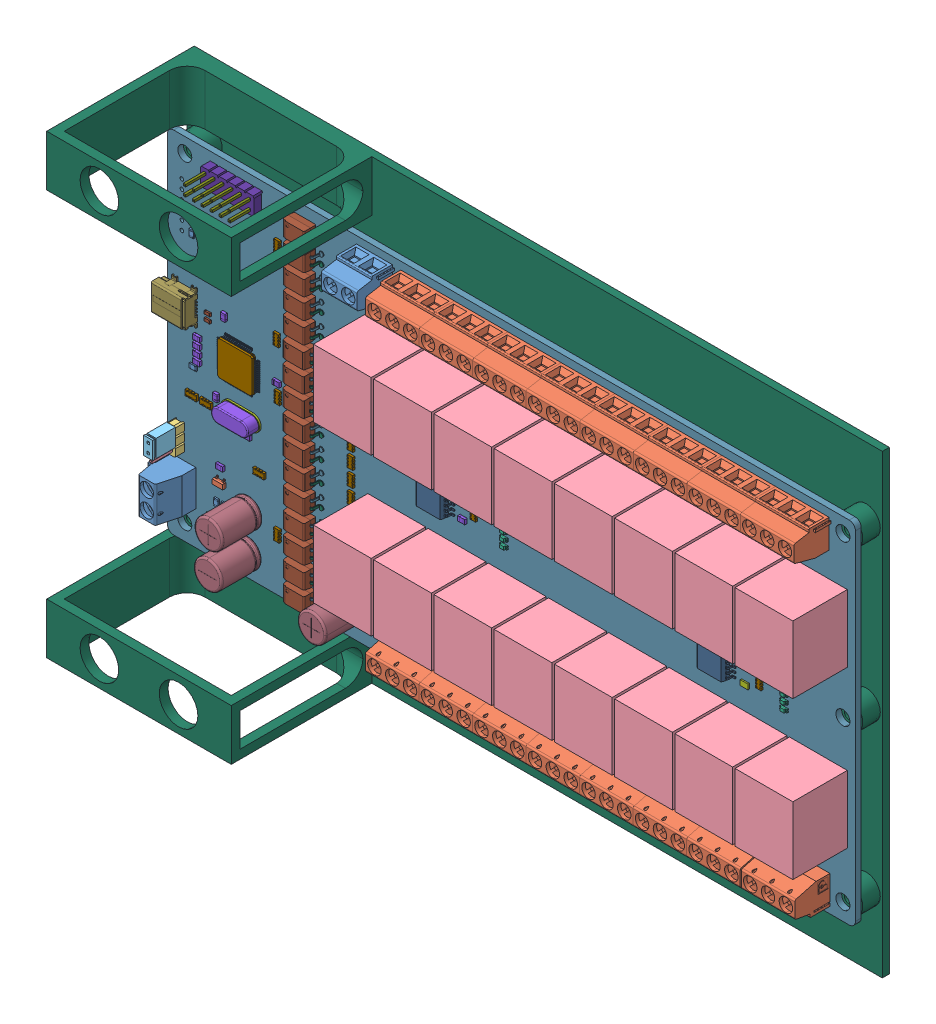
SolidWorks assembly Assem2, configuration Default. Lengths in mm.
Overall size (201.04 129.82 42).
600 component instances, 33 part files, 0 mates.
Components (placement in the parent):
- 16_Channel_USB_Relay.step-1: 16_Channel_USB_Relay.step [Default] at (-11.9082 58.988 141.1455) size (200.04 103.47 20)
  - X277.step-1: X277.step [Default] at origin size (10.73 8.1 13.5)
    - 1729128_07.step-1: 1729128_07.step [Default] at (64.7474 97.3538 0) x (0 1 0) z (1 0 0) size (8.1 13.5 10.73)
      - mkdsn_1.5-2-5.08.step-1: mkdsn_1.5-2-5.08.step [Default] at (-39.331 -15.5089 -8.19) x (-1 0 0) z (0 0 -1) size (8.1 13.5 10.73)
  - X276.step-1: X276.step [Default] at origin size (15.81 8.1 13.5)
    - 1729131_07.step-1: 1729131_07.step [Default] at (173.1033 2.7699 0.1541) x (0 -1 0) z (-1 0 0) size (8.1 13.5 15.81)
      - mkdsn_1.5-3-5.08.step-1: mkdsn_1.5-3-5.08.step [Default] at (-39.331 -15.5089 -8.19) x (-1 0 0) z (0 0 -1) size (8.1 13.5 15.81)
  - X275.step-1: X275.step [Default] at origin size (15.81 8.1 13.5)
    - 1729131_07.step-1: 1729131_07.step [Default] at (157.5733 2.7699 0.1541) x (0 -1 0) z (-1 0 0) size (8.1 13.5 15.81)
      - mkdsn_1.5-3-5.08.step-1: mkdsn_1.5-3-5.08.step [Default] at (-39.331 -15.5089 -8.19) x (-1 0 0) z (0 0 -1) size (8.1 13.5 15.81)
  - X274.step-1: X274.step [Default] at origin size (15.81 8.1 13.5)
    - 1729131_07.step-1: 1729131_07.step [Default] at (142.3333 2.7699 0.1541) x (0 -1 0) z (-1 0 0) size (8.1 13.5 15.81)
      - mkdsn_1.5-3-5.08.step-1: mkdsn_1.5-3-5.08.step [Default] at (-39.331 -15.5089 -8.19) x (-1 0 0) z (0 0 -1) size (8.1 13.5 15.81)
  - X273.step-1: X273.step [Default] at origin size (15.81 8.1 13.5)
    - 1729131_07.step-1: 1729131_07.step [Default] at (127.0933 2.7699 0.1541) x (0 -1 0) z (-1 0 0) size (8.1 13.5 15.81)
      - mkdsn_1.5-3-5.08.step-1: mkdsn_1.5-3-5.08.step [Default] at (-39.331 -15.5089 -8.19) x (-1 0 0) z (0 0 -1) size (8.1 13.5 15.81)
  - X272.step-1: X272.step [Default] at origin size (15.81 8.1 13.5)
    - 1729131_07.step-1: 1729131_07.step [Default] at (111.8533 2.7699 0.1541) x (0 -1 0) z (-1 0 0) size (8.1 13.5 15.81)
      - mkdsn_1.5-3-5.08.step-1: mkdsn_1.5-3-5.08.step [Default] at (-39.331 -15.5089 -8.19) x (-1 0 0) z (0 0 -1) size (8.1 13.5 15.81)
  - X271.step-1: X271.step [Default] at origin size (15.81 8.1 13.5)
    - 1729131_07.step-1: 1729131_07.step [Default] at (96.6133 2.7699 0.1541) x (0 -1 0) z (-1 0 0) size (8.1 13.5 15.81)
      - mkdsn_1.5-3-5.08.step-1: mkdsn_1.5-3-5.08.step [Default] at (-39.331 -15.5089 -8.19) x (-1 0 0) z (0 0 -1) size (8.1 13.5 15.81)
  - X270.step-1: X270.step [Default] at origin size (15.81 8.1 13.5)
    - 1729131_07.step-1: 1729131_07.step [Default] at (81.3733 2.7699 0.1541) x (0 -1 0) z (-1 0 0) size (8.1 13.5 15.81)
      - mkdsn_1.5-3-5.08.step-1: mkdsn_1.5-3-5.08.step [Default] at (-39.331 -15.5089 -8.19) x (-1 0 0) z (0 0 -1) size (8.1 13.5 15.81)
  - X269.step-1: X269.step [Default] at origin size (15.81 8.1 13.5)
    - 1729131_07.step-1: 1729131_07.step [Default] at (66.1333 2.7699 0.1541) x (0 -1 0) z (-1 0 0) size (8.1 13.5 15.81)
      - mkdsn_1.5-3-5.08.step-1: mkdsn_1.5-3-5.08.step [Default] at (-39.331 -15.5089 -8.19) x (-1 0 0) z (0 0 -1) size (8.1 13.5 15.81)
  - X268.step-1: X268.step [Default] at origin size (15.81 8.1 13.5)
    - 1729131_07.step-1: 1729131_07.step [Default] at (189.2327 97.3821 0.1541) x (0 1 0) z (1 0 0) size (8.1 13.5 15.81)
      - mkdsn_1.5-3-5.08.step-1: mkdsn_1.5-3-5.08.step [Default] at (-39.331 -15.5089 -8.19) x (-1 0 0) z (0 0 -1) size (8.1 13.5 15.81)
  - X267.step-1: X267.step [Default] at origin size (15.81 8.1 13.5)
    - 1729131_07.step-1: 1729131_07.step [Default] at (173.9927 97.3821 0.1541) x (0 1 0) z (1 0 0) size (8.1 13.5 15.81)
      - mkdsn_1.5-3-5.08.step-1: mkdsn_1.5-3-5.08.step [Default] at (-39.331 -15.5089 -8.19) x (-1 0 0) z (0 0 -1) size (8.1 13.5 15.81)
  - X266.step-1: X266.step [Default] at origin size (15.81 8.1 13.5)
    - 1729131_07.step-1: 1729131_07.step [Default] at (158.7527 97.3821 0.1541) x (0 1 0) z (1 0 0) size (8.1 13.5 15.81)
      - mkdsn_1.5-3-5.08.step-1: mkdsn_1.5-3-5.08.step [Default] at (-39.331 -15.5089 -8.19) x (-1 0 0) z (0 0 -1) size (8.1 13.5 15.81)
  - X265.step-1: X265.step [Default] at origin size (15.81 8.1 13.5)
    - 1729131_07.step-1: 1729131_07.step [Default] at (143.5127 97.3821 0.1541) x (0 1 0) z (1 0 0) size (8.1 13.5 15.81)
      - mkdsn_1.5-3-5.08.step-1: mkdsn_1.5-3-5.08.step [Default] at (-39.331 -15.5089 -8.19) x (-1 0 0) z (0 0 -1) size (8.1 13.5 15.81)
  - X264.step-1: X264.step [Default] at origin size (15.81 8.1 13.5)
    - 1729131_07.step-1: 1729131_07.step [Default] at (128.2727 97.3821 0.1541) x (0 1 0) z (1 0 0) size (8.1 13.5 15.81)
      - mkdsn_1.5-3-5.08.step-1: mkdsn_1.5-3-5.08.step [Default] at (-39.331 -15.5089 -8.19) x (-1 0 0) z (0 0 -1) size (8.1 13.5 15.81)
  - X263.step-1: X263.step [Default] at origin size (15.81 8.1 13.5)
    - 1729131_07.step-1: 1729131_07.step [Default] at (113.0327 97.3821 0.1541) x (0 1 0) z (1 0 0) size (8.1 13.5 15.81)
      - mkdsn_1.5-3-5.08.step-1: mkdsn_1.5-3-5.08.step [Default] at (-39.331 -15.5089 -8.19) x (-1 0 0) z (0 0 -1) size (8.1 13.5 15.81)
  - X262.step-1: X262.step [Default] at origin size (15.81 8.1 13.5)
    - 1729131_07.step-1: 1729131_07.step [Default] at (97.7927 97.3821 0.1541) x (0 1 0) z (1 0 0) size (8.1 13.5 15.81)
      - mkdsn_1.5-3-5.08.step-1: mkdsn_1.5-3-5.08.step [Default] at (-39.331 -15.5089 -8.19) x (-1 0 0) z (0 0 -1) size (8.1 13.5 15.81)
  - X261.step-1: X261.step [Default] at origin size (15.81 8.1 13.5)
    - 1729131_07.step-1: 1729131_07.step [Default] at (82.5527 97.3821 0.1541) x (0 1 0) z (1 0 0) size (8.1 13.5 15.81)
      - mkdsn_1.5-3-5.08.step-1: mkdsn_1.5-3-5.08.step [Default] at (-39.331 -15.5089 -8.19) x (-1 0 0) z (0 0 -1) size (8.1 13.5 15.81)
  - X260.step-1: X260.step [Default] at origin size (16.46 19.18 20)
    - 503707232.step-1: 503707232.step [Default] at (191.3354 21.8311 0) x (0 -1 0) z (0 0 -1) size (0.4 0.4 4.5)
      - Cylinder.step-1: Cylinder.step [Default] at origin size (0.4 0.4 4.5)
    - 503707232.step-2: 503707232.step [Default] at (191.3354 33.7691 0) x (0 -1 0) z (0 0 -1) size (0.4 0.4 4.5)
      - Cylinder.step-1: Cylinder.step [Default] at origin size (0.4 0.4 4.5)
    - 503707232.step-3: 503707232.step [Default] at (185.3665 36.0551 0) x (0 -1 0) z (0 0 -1) size (0.4 0.4 4.5)
      - Cylinder.step-1: Cylinder.step [Default] at origin size (0.4 0.4 4.5)
    - 503707232.step-4: 503707232.step [Default] at (179.3974 33.7691 0) x (0 -1 0) z (0 0 -1) size (0.4 0.4 4.5)
      - Cylinder.step-1: Cylinder.step [Default] at origin size (0.4 0.4 4.5)
    - 503707232.step-5: 503707232.step [Default] at (179.3974 21.8311 0) x (0 -1 0) z (0 0 -1) size (0.4 0.4 4.5)
      - Cylinder.step-1: Cylinder.step [Default] at origin size (0.4 0.4 4.5)
    - 541420192.step-1: 541420192.step [Default] at (185.468 28.4225 0) size (16.46 19.18 15.5)
      - Extruded.step-1: Extruded.step [Default] at origin size (16.46 19.18 15.5)
  - X259.step-1: X259.step [Default] at origin size (16.46 19.18 20)
    - 541420192.step-1: 541420192.step [Default] at (168.323 28.4225 0) size (16.46 19.18 15.5)
      - Extruded.step-1: Extruded.step [Default] at origin size (16.46 19.18 15.5)
    - 503707232.step-1: 503707232.step [Default] at (162.2524 21.8311 0) x (0 -1 0) z (0 0 -1) size (0.4 0.4 4.5)
      - Cylinder.step-1: Cylinder.step [Default] at origin size (0.4 0.4 4.5)
    - 503707232.step-2: 503707232.step [Default] at (162.2524 33.7691 0) x (0 -1 0) z (0 0 -1) size (0.4 0.4 4.5)
      - Cylinder.step-1: Cylinder.step [Default] at origin size (0.4 0.4 4.5)
    - 503707232.step-3: 503707232.step [Default] at (168.2214 36.0551 0) x (0 -1 0) z (0 0 -1) size (0.4 0.4 4.5)
      - Cylinder.step-1: Cylinder.step [Default] at origin size (0.4 0.4 4.5)
    - 503707232.step-4: 503707232.step [Default] at (174.1904 33.7691 0) x (0 -1 0) z (0 0 -1) size (0.4 0.4 4.5)
      - Cylinder.step-1: Cylinder.step [Default] at origin size (0.4 0.4 4.5)
    - 503707232.step-5: 503707232.step [Default] at (174.1904 21.8311 0) x (0 -1 0) z (0 0 -1) size (0.4 0.4 4.5)
      - Cylinder.step-1: Cylinder.step [Default] at origin size (0.4 0.4 4.5)
  - X258.step-1: X258.step [Default] at origin size (16.46 19.18 20)
    - 503707232.step-1: 503707232.step [Default] at (157.0454 21.8311 0) x (0 -1 0) z (0 0 -1) size (0.4 0.4 4.5)
      - Cylinder.step-1: Cylinder.step [Default] at origin size (0.4 0.4 4.5)
    - 503707232.step-2: 503707232.step [Default] at (157.0454 33.7691 0) x (0 -1 0) z (0 0 -1) size (0.4 0.4 4.5)
      - Cylinder.step-1: Cylinder.step [Default] at origin size (0.4 0.4 4.5)
    - 503707232.step-3: 503707232.step [Default] at (151.0764 36.0551 0) x (0 -1 0) z (0 0 -1) size (0.4 0.4 4.5)
      - Cylinder.step-1: Cylinder.step [Default] at origin size (0.4 0.4 4.5)
    - 503707232.step-4: 503707232.step [Default] at (145.1074 33.7691 0) x (0 -1 0) z (0 0 -1) size (0.4 0.4 4.5)
      - Cylinder.step-1: Cylinder.step [Default] at origin size (0.4 0.4 4.5)
    - 503707232.step-5: 503707232.step [Default] at (145.1074 21.8311 0) x (0 -1 0) z (0 0 -1) size (0.4 0.4 4.5)
      - Cylinder.step-1: Cylinder.step [Default] at origin size (0.4 0.4 4.5)
    - 541420192.step-1: 541420192.step [Default] at (151.178 28.4225 0) size (16.46 19.18 15.5)
      - Extruded.step-1: Extruded.step [Default] at origin size (16.46 19.18 15.5)
  - X257.step-1: X257.step [Default] at origin size (16.46 19.18 20)
    - 541420192.step-1: 541420192.step [Default] at (134.033 28.4225 0) size (16.46 19.18 15.5)
      - Extruded.step-1: Extruded.step [Default] at origin size (16.46 19.18 15.5)
    - 503707232.step-1: 503707232.step [Default] at (127.9624 21.8311 0) x (0 -1 0) z (0 0 -1) size (0.4 0.4 4.5)
      - Cylinder.step-1: Cylinder.step [Default] at origin size (0.4 0.4 4.5)
    - 503707232.step-2: 503707232.step [Default] at (127.9624 33.7691 0) x (0 -1 0) z (0 0 -1) size (0.4 0.4 4.5)
      - Cylinder.step-1: Cylinder.step [Default] at origin size (0.4 0.4 4.5)
    - 503707232.step-3: 503707232.step [Default] at (133.9314 36.0551 0) x (0 -1 0) z (0 0 -1) size (0.4 0.4 4.5)
      - Cylinder.step-1: Cylinder.step [Default] at origin size (0.4 0.4 4.5)
    - 503707232.step-4: 503707232.step [Default] at (139.9004 33.7691 0) x (0 -1 0) z (0 0 -1) size (0.4 0.4 4.5)
      - Cylinder.step-1: Cylinder.step [Default] at origin size (0.4 0.4 4.5)
    - 503707232.step-5: 503707232.step [Default] at (139.9004 21.8311 0) x (0 -1 0) z (0 0 -1) size (0.4 0.4 4.5)
      - Cylinder.step-1: Cylinder.step [Default] at origin size (0.4 0.4 4.5)
  - X256.step-1: X256.step [Default] at origin size (16.46 19.18 20)
    - 503707232.step-1: 503707232.step [Default] at (122.7554 21.8311 0) x (0 -1 0) z (0 0 -1) size (0.4 0.4 4.5)
      - Cylinder.step-1: Cylinder.step [Default] at origin size (0.4 0.4 4.5)
    - 503707232.step-2: 503707232.step [Default] at (122.7554 33.7691 0) x (0 -1 0) z (0 0 -1) size (0.4 0.4 4.5)
      - Cylinder.step-1: Cylinder.step [Default] at origin size (0.4 0.4 4.5)
    - 503707232.step-3: 503707232.step [Default] at (116.7864 36.0551 0) x (0 -1 0) z (0 0 -1) size (0.4 0.4 4.5)
      - Cylinder.step-1: Cylinder.step [Default] at origin size (0.4 0.4 4.5)
    - 503707232.step-4: 503707232.step [Default] at (110.8174 33.7691 0) x (0 -1 0) z (0 0 -1) size (0.4 0.4 4.5)
      - Cylinder.step-1: Cylinder.step [Default] at origin size (0.4 0.4 4.5)
    - 503707232.step-5: 503707232.step [Default] at (110.8174 21.8311 0) x (0 -1 0) z (0 0 -1) size (0.4 0.4 4.5)
      - Cylinder.step-1: Cylinder.step [Default] at origin size (0.4 0.4 4.5)
    - 541420192.step-1: 541420192.step [Default] at (116.888 28.4225 0) size (16.46 19.18 15.5)
      - Extruded.step-1: Extruded.step [Default] at origin size (16.46 19.18 15.5)
  - X255.step-1: X255.step [Default] at origin size (16.46 19.18 20)
    - 541420192.step-1: 541420192.step [Default] at (99.743 28.4225 0) size (16.46 19.18 15.5)
      - Extruded.step-1: Extruded.step [Default] at origin size (16.46 19.18 15.5)
    - 503707232.step-1: 503707232.step [Default] at (93.6724 21.8311 0) x (0 -1 0) z (0 0 -1) size (0.4 0.4 4.5)
      - Cylinder.step-1: Cylinder.step [Default] at origin size (0.4 0.4 4.5)
    - 503707232.step-2: 503707232.step [Default] at (93.6724 33.7691 0) x (0 -1 0) z (0 0 -1) size (0.4 0.4 4.5)
      - Cylinder.step-1: Cylinder.step [Default] at origin size (0.4 0.4 4.5)
    - 503707232.step-3: 503707232.step [Default] at (99.6414 36.0551 0) x (0 -1 0) z (0 0 -1) size (0.4 0.4 4.5)
      - Cylinder.step-1: Cylinder.step [Default] at origin size (0.4 0.4 4.5)
    - 503707232.step-4: 503707232.step [Default] at (105.6104 33.7691 0) x (0 -1 0) z (0 0 -1) size (0.4 0.4 4.5)
      - Cylinder.step-1: Cylinder.step [Default] at origin size (0.4 0.4 4.5)
    - 503707232.step-5: 503707232.step [Default] at (105.6104 21.8311 0) x (0 -1 0) z (0 0 -1) size (0.4 0.4 4.5)
      - Cylinder.step-1: Cylinder.step [Default] at origin size (0.4 0.4 4.5)
  - X254.step-1: X254.step [Default] at origin size (16.46 19.18 20)
    - 503707232.step-1: 503707232.step [Default] at (88.4654 21.8311 0) x (0 -1 0) z (0 0 -1) size (0.4 0.4 4.5)
      - Cylinder.step-1: Cylinder.step [Default] at origin size (0.4 0.4 4.5)
    - 503707232.step-2: 503707232.step [Default] at (88.4654 33.7691 0) x (0 -1 0) z (0 0 -1) size (0.4 0.4 4.5)
      - Cylinder.step-1: Cylinder.step [Default] at origin size (0.4 0.4 4.5)
    - 503707232.step-3: 503707232.step [Default] at (82.4964 36.0551 0) x (0 -1 0) z (0 0 -1) size (0.4 0.4 4.5)
      - Cylinder.step-1: Cylinder.step [Default] at origin size (0.4 0.4 4.5)
    - 503707232.step-4: 503707232.step [Default] at (76.5274 33.7691 0) x (0 -1 0) z (0 0 -1) size (0.4 0.4 4.5)
      - Cylinder.step-1: Cylinder.step [Default] at origin size (0.4 0.4 4.5)
    - 503707232.step-5: 503707232.step [Default] at (76.5274 21.8311 0) x (0 -1 0) z (0 0 -1) size (0.4 0.4 4.5)
      - Cylinder.step-1: Cylinder.step [Default] at origin size (0.4 0.4 4.5)
    - 541420192.step-1: 541420192.step [Default] at (82.598 28.4225 0) size (16.46 19.18 15.5)
      - Extruded.step-1: Extruded.step [Default] at origin size (16.46 19.18 15.5)
  - X253.step-1: X253.step [Default] at origin size (16.46 19.18 20)
    - 541420192.step-1: 541420192.step [Default] at (65.453 28.4225 0) size (16.46 19.18 15.5)
      - Extruded.step-1: Extruded.step [Default] at origin size (16.46 19.18 15.5)
    - 503707232.step-1: 503707232.step [Default] at (59.3824 21.8311 0) x (0 -1 0) z (0 0 -1) size (0.4 0.4 4.5)
      - Cylinder.step-1: Cylinder.step [Default] at origin size (0.4 0.4 4.5)
    - 503707232.step-2: 503707232.step [Default] at (59.3824 33.7691 0) x (0 -1 0) z (0 0 -1) size (0.4 0.4 4.5)
      - Cylinder.step-1: Cylinder.step [Default] at origin size (0.4 0.4 4.5)
    - 503707232.step-3: 503707232.step [Default] at (65.3514 36.0551 0) x (0 -1 0) z (0 0 -1) size (0.4 0.4 4.5)
      - Cylinder.step-1: Cylinder.step [Default] at origin size (0.4 0.4 4.5)
    - 503707232.step-4: 503707232.step [Default] at (71.3204 33.7691 0) x (0 -1 0) z (0 0 -1) size (0.4 0.4 4.5)
      - Cylinder.step-1: Cylinder.step [Default] at origin size (0.4 0.4 4.5)
    - 503707232.step-5: 503707232.step [Default] at (71.3204 21.8311 0) x (0 -1 0) z (0 0 -1) size (0.4 0.4 4.5)
      - Cylinder.step-1: Cylinder.step [Default] at origin size (0.4 0.4 4.5)
  - X252.step-1: X252.step [Default] at origin size (16.46 19.18 20)
    - 753223104.step-1: 753223104.step [Default] at (59.5856 79.5909 0) x (0 1 0) z (0 0 -1) size (0.4 0.4 4.5)
      - Cylinder-0.step-1: Cylinder-0.step [Default] at origin size (0.4 0.4 4.5)
    - 753223104.step-2: 753223104.step [Default] at (59.5856 67.6529 0) x (0 1 0) z (0 0 -1) size (0.4 0.4 4.5)
      - Cylinder-0.step-1: Cylinder-0.step [Default] at origin size (0.4 0.4 4.5)
    - 753223104.step-3: 753223104.step [Default] at (65.5546 65.3669 0) x (0 1 0) z (0 0 -1) size (0.4 0.4 4.5)
      - Cylinder-0.step-1: Cylinder-0.step [Default] at origin size (0.4 0.4 4.5)
    - 753223104.step-4: 753223104.step [Default] at (71.5236 67.6529 0) x (0 1 0) z (0 0 -1) size (0.4 0.4 4.5)
      - Cylinder-0.step-1: Cylinder-0.step [Default] at origin size (0.4 0.4 4.5)
    - 753223104.step-5: 753223104.step [Default] at (71.5236 79.5909 0) x (0 1 0) z (0 0 -1) size (0.4 0.4 4.5)
      - Cylinder-0.step-1: Cylinder-0.step [Default] at origin size (0.4 0.4 4.5)
    - 541420192.step-1: 541420192.step [Default] at (65.453 72.9995 0) size (16.46 19.18 15.5)
      - Extruded.step-1: Extruded.step [Default] at origin size (16.46 19.18 15.5)
  - X251.step-1: X251.step [Default] at origin size (16.46 19.18 20)
    - 541420192.step-1: 541420192.step [Default] at (82.598 72.9995 0) size (16.46 19.18 15.5)
      - Extruded.step-1: Extruded.step [Default] at origin size (16.46 19.18 15.5)
    - 753223104.step-1: 753223104.step [Default] at (88.6686 79.5909 0) x (0 1 0) z (0 0 -1) size (0.4 0.4 4.5)
      - Cylinder-0.step-1: Cylinder-0.step [Default] at origin size (0.4 0.4 4.5)
    - 753223104.step-2: 753223104.step [Default] at (88.6686 67.6529 0) x (0 1 0) z (0 0 -1) size (0.4 0.4 4.5)
      - Cylinder-0.step-1: Cylinder-0.step [Default] at origin size (0.4 0.4 4.5)
    - 753223104.step-3: 753223104.step [Default] at (82.6996 65.3669 0) x (0 1 0) z (0 0 -1) size (0.4 0.4 4.5)
      - Cylinder-0.step-1: Cylinder-0.step [Default] at origin size (0.4 0.4 4.5)
    - 753223104.step-4: 753223104.step [Default] at (76.7306 67.6529 0) x (0 1 0) z (0 0 -1) size (0.4 0.4 4.5)
      - Cylinder-0.step-1: Cylinder-0.step [Default] at origin size (0.4 0.4 4.5)
    - 753223104.step-5: 753223104.step [Default] at (76.7306 79.5909 0) x (0 1 0) z (0 0 -1) size (0.4 0.4 4.5)
      - Cylinder-0.step-1: Cylinder-0.step [Default] at origin size (0.4 0.4 4.5)
  - X250.step-1: X250.step [Default] at origin size (16.46 19.18 20)
    - 753223104.step-1: 753223104.step [Default] at (93.8756 79.5909 0) x (0 1 0) z (0 0 -1) size (0.4 0.4 4.5)
      - Cylinder-0.step-1: Cylinder-0.step [Default] at origin size (0.4 0.4 4.5)
    - 753223104.step-2: 753223104.step [Default] at (93.8756 67.6529 0) x (0 1 0) z (0 0 -1) size (0.4 0.4 4.5)
      - Cylinder-0.step-1: Cylinder-0.step [Default] at origin size (0.4 0.4 4.5)
    - 753223104.step-3: 753223104.step [Default] at (99.8446 65.3669 0) x (0 1 0) z (0 0 -1) size (0.4 0.4 4.5)
      - Cylinder-0.step-1: Cylinder-0.step [Default] at origin size (0.4 0.4 4.5)
    - 753223104.step-4: 753223104.step [Default] at (105.8136 67.6529 0) x (0 1 0) z (0 0 -1) size (0.4 0.4 4.5)
      - Cylinder-0.step-1: Cylinder-0.step [Default] at origin size (0.4 0.4 4.5)
    - 753223104.step-5: 753223104.step [Default] at (105.8136 79.5909 0) x (0 1 0) z (0 0 -1) size (0.4 0.4 4.5)
      - Cylinder-0.step-1: Cylinder-0.step [Default] at origin size (0.4 0.4 4.5)
    - 541420192.step-1: 541420192.step [Default] at (99.743 72.9995 0) size (16.46 19.18 15.5)
      - Extruded.step-1: Extruded.step [Default] at origin size (16.46 19.18 15.5)
  - X249.step-1: X249.step [Default] at origin size (16.46 19.18 20)
    - 541420192.step-1: 541420192.step [Default] at (116.888 72.9995 0) size (16.46 19.18 15.5)
      - Extruded.step-1: Extruded.step [Default] at origin size (16.46 19.18 15.5)
    - 753223104.step-1: 753223104.step [Default] at (122.9586 79.5909 0) x (0 1 0) z (0 0 -1) size (0.4 0.4 4.5)
      - Cylinder-0.step-1: Cylinder-0.step [Default] at origin size (0.4 0.4 4.5)
    - 753223104.step-2: 753223104.step [Default] at (122.9586 67.6529 0) x (0 1 0) z (0 0 -1) size (0.4 0.4 4.5)
      - Cylinder-0.step-1: Cylinder-0.step [Default] at origin size (0.4 0.4 4.5)
    - 753223104.step-3: 753223104.step [Default] at (116.9896 65.3669 0) x (0 1 0) z (0 0 -1) size (0.4 0.4 4.5)
      - Cylinder-0.step-1: Cylinder-0.step [Default] at origin size (0.4 0.4 4.5)
    - 753223104.step-4: 753223104.step [Default] at (111.0206 67.6529 0) x (0 1 0) z (0 0 -1) size (0.4 0.4 4.5)
      - Cylinder-0.step-1: Cylinder-0.step [Default] at origin size (0.4 0.4 4.5)
    - 753223104.step-5: 753223104.step [Default] at (111.0206 79.5909 0) x (0 1 0) z (0 0 -1) size (0.4 0.4 4.5)
      - Cylinder-0.step-1: Cylinder-0.step [Default] at origin size (0.4 0.4 4.5)
  - X248.step-1: X248.step [Default] at origin size (16.46 19.18 20)
    - 753223104.step-1: 753223104.step [Default] at (128.1656 79.5909 0) x (0 1 0) z (0 0 -1) size (0.4 0.4 4.5)
      - Cylinder-0.step-1: Cylinder-0.step [Default] at origin size (0.4 0.4 4.5)
    - 753223104.step-2: 753223104.step [Default] at (128.1656 67.6529 0) x (0 1 0) z (0 0 -1) size (0.4 0.4 4.5)
      - Cylinder-0.step-1: Cylinder-0.step [Default] at origin size (0.4 0.4 4.5)
    - 753223104.step-3: 753223104.step [Default] at (134.1346 65.3669 0) x (0 1 0) z (0 0 -1) size (0.4 0.4 4.5)
      - Cylinder-0.step-1: Cylinder-0.step [Default] at origin size (0.4 0.4 4.5)
    - 753223104.step-4: 753223104.step [Default] at (140.1036 67.6529 0) x (0 1 0) z (0 0 -1) size (0.4 0.4 4.5)
      - Cylinder-0.step-1: Cylinder-0.step [Default] at origin size (0.4 0.4 4.5)
    - 753223104.step-5: 753223104.step [Default] at (140.1036 79.5909 0) x (0 1 0) z (0 0 -1) size (0.4 0.4 4.5)
      - Cylinder-0.step-1: Cylinder-0.step [Default] at origin size (0.4 0.4 4.5)
    - 541420192.step-1: 541420192.step [Default] at (134.033 72.9995 0) size (16.46 19.18 15.5)
      - Extruded.step-1: Extruded.step [Default] at origin size (16.46 19.18 15.5)
  - X247.step-1: X247.step [Default] at origin size (16.46 19.18 20)
    - 541420192.step-1: 541420192.step [Default] at (151.178 72.9995 0) size (16.46 19.18 15.5)
      - Extruded.step-1: Extruded.step [Default] at origin size (16.46 19.18 15.5)
    - 753223104.step-1: 753223104.step [Default] at (157.2486 79.5909 0) x (0 1 0) z (0 0 -1) size (0.4 0.4 4.5)
      - Cylinder-0.step-1: Cylinder-0.step [Default] at origin size (0.4 0.4 4.5)
    - 753223104.step-2: 753223104.step [Default] at (157.2486 67.6529 0) x (0 1 0) z (0 0 -1) size (0.4 0.4 4.5)
      - Cylinder-0.step-1: Cylinder-0.step [Default] at origin size (0.4 0.4 4.5)
    - 753223104.step-3: 753223104.step [Default] at (151.2796 65.3669 0) x (0 1 0) z (0 0 -1) size (0.4 0.4 4.5)
      - Cylinder-0.step-1: Cylinder-0.step [Default] at origin size (0.4 0.4 4.5)
    - 753223104.step-4: 753223104.step [Default] at (145.3106 67.6529 0) x (0 1 0) z (0 0 -1) size (0.4 0.4 4.5)
      - Cylinder-0.step-1: Cylinder-0.step [Default] at origin size (0.4 0.4 4.5)
    - 753223104.step-5: 753223104.step [Default] at (145.3106 79.5909 0) x (0 1 0) z (0 0 -1) size (0.4 0.4 4.5)
      - Cylinder-0.step-1: Cylinder-0.step [Default] at origin size (0.4 0.4 4.5)
  - X246.step-1: X246.step [Default] at origin size (16.46 19.18 20)
    - 753223104.step-1: 753223104.step [Default] at (162.4556 79.5909 0) x (0 1 0) z (0 0 -1) size (0.4 0.4 4.5)
      - Cylinder-0.step-1: Cylinder-0.step [Default] at origin size (0.4 0.4 4.5)
    - 753223104.step-2: 753223104.step [Default] at (162.4556 67.6529 0) x (0 1 0) z (0 0 -1) size (0.4 0.4 4.5)
      - Cylinder-0.step-1: Cylinder-0.step [Default] at origin size (0.4 0.4 4.5)
    - 753223104.step-3: 753223104.step [Default] at (168.4246 65.3669 0) x (0 1 0) z (0 0 -1) size (0.4 0.4 4.5)
      - Cylinder-0.step-1: Cylinder-0.step [Default] at origin size (0.4 0.4 4.5)
    - 753223104.step-4: 753223104.step [Default] at (174.3936 67.6529 0) x (0 1 0) z (0 0 -1) size (0.4 0.4 4.5)
      - Cylinder-0.step-1: Cylinder-0.step [Default] at origin size (0.4 0.4 4.5)
    - 753223104.step-5: 753223104.step [Default] at (174.3936 79.5909 0) x (0 1 0) z (0 0 -1) size (0.4 0.4 4.5)
      - Cylinder-0.step-1: Cylinder-0.step [Default] at origin size (0.4 0.4 4.5)
    - 541420192.step-1: 541420192.step [Default] at (168.323 72.9995 0) size (16.46 19.18 15.5)
      - Extruded.step-1: Extruded.step [Default] at origin size (16.46 19.18 15.5)
  - X245.step-1: X245.step [Default] at origin size (16.46 19.18 20)
    - 541420192.step-1: 541420192.step [Default] at (185.468 72.9995 0) size (16.46 19.18 15.5)
      - Extruded.step-1: Extruded.step [Default] at origin size (16.46 19.18 15.5)
    - 753223104.step-1: 753223104.step [Default] at (191.5386 79.5909 0) x (0 1 0) z (0 0 -1) size (0.4 0.4 4.5)
      - Cylinder-0.step-1: Cylinder-0.step [Default] at origin size (0.4 0.4 4.5)
    - 753223104.step-2: 753223104.step [Default] at (191.5386 67.6529 0) x (0 1 0) z (0 0 -1) size (0.4 0.4 4.5)
      - Cylinder-0.step-1: Cylinder-0.step [Default] at origin size (0.4 0.4 4.5)
    - 753223104.step-3: 753223104.step [Default] at (185.5695 65.3669 0) x (0 1 0) z (0 0 -1) size (0.4 0.4 4.5)
      - Cylinder-0.step-1: Cylinder-0.step [Default] at origin size (0.4 0.4 4.5)
    - 753223104.step-4: 753223104.step [Default] at (179.6006 67.6529 0) x (0 1 0) z (0 0 -1) size (0.4 0.4 4.5)
      - Cylinder-0.step-1: Cylinder-0.step [Default] at origin size (0.4 0.4 4.5)
    - 753223104.step-5: 753223104.step [Default] at (179.6006 79.5909 0) x (0 1 0) z (0 0 -1) size (0.4 0.4 4.5)
      - Cylinder-0.step-1: Cylinder-0.step [Default] at origin size (0.4 0.4 4.5)
  - D9.step-1: D9.step [Default] at origin size (2.06 0.91 0.84)
    - SW3dPS-LED_SMD0805.step-1: SW3dPS-LED_SMD0805.step [Default] at (176.7045 44.3798 0) x (0 -1 0) z (0 0 1) size (0.91 2.06 0.84)
  - D8.step-1: D8.step [Default] at origin size (2.06 0.91 0.84)
    - SW3dPS-LED_SMD0805.step-1: SW3dPS-LED_SMD0805.step [Default] at (176.7045 46.2848 0) x (0 -1 0) z (0 0 1) size (0.91 2.06 0.84)
  - D7.step-1: D7.step [Default] at origin size (2.06 0.91 0.84)
    - SW3dPS-LED_SMD0805.step-1: SW3dPS-LED_SMD0805.step [Default] at (176.7045 48.1898 0) x (0 -1 0) z (0 0 1) size (0.91 2.06 0.84)
  - D6.step-1: D6.step [Default] at origin size (2.06 0.91 0.84)
    - SW3dPS-LED_SMD0805.step-1: SW3dPS-LED_SMD0805.step [Default] at (176.7045 50.0948 0) x (0 -1 0) z (0 0 1) size (0.91 2.06 0.84)
  - D5.step-1: D5.step [Default] at origin size (2.06 0.91 0.84)
    - SW3dPS-LED_SMD0805.step-1: SW3dPS-LED_SMD0805.step [Default] at (176.7045 51.9998 0) x (0 -1 0) z (0 0 1) size (0.91 2.06 0.84)
  - D4.step-1: D4.step [Default] at origin size (2.06 0.91 0.84)
    - SW3dPS-LED_SMD0805.step-1: SW3dPS-LED_SMD0805.step [Default] at (176.7045 53.9048 0) x (0 -1 0) z (0 0 1) size (0.91 2.06 0.84)
  - D3.step-1: D3.step [Default] at origin size (2.06 0.91 0.84)
    - SW3dPS-LED_SMD0805.step-1: SW3dPS-LED_SMD0805.step [Default] at (176.7045 55.8098 0) x (0 -1 0) z (0 0 1) size (0.91 2.06 0.84)
  - D2.step-1: D2.step [Default] at origin size (2.06 0.91 0.84)
    - SW3dPS-LED_SMD0805.step-1: SW3dPS-LED_SMD0805.step [Default] at (176.7045 57.7148 0) x (0 -1 0) z (0 0 1) size (0.91 2.06 0.84)
  - D13.step-1: D13.step [Default] at origin size (2.06 0.91 0.84)
    - SW3dPS-LED_SMD0805.step-1: SW3dPS-LED_SMD0805.step [Default] at (96.9612 44.6592 0) x (0 -1 0) z (0 0 1) size (0.91 2.06 0.84)
  - D12.step-1: D12.step [Default] at origin size (2.06 0.91 0.84)
    - SW3dPS-LED_SMD0805.step-1: SW3dPS-LED_SMD0805.step [Default] at (96.9612 46.5642 0) x (0 -1 0) z (0 0 1) size (0.91 2.06 0.84)
  - D11.step-1: D11.step [Default] at origin size (2.06 0.91 0.84)
    - SW3dPS-LED_SMD0805.step-1: SW3dPS-LED_SMD0805.step [Default] at (96.9612 48.4438 0) x (0 -1 0) z (0 0 1) size (0.91 2.06 0.84)
  - D10.step-1: D10.step [Default] at origin size (2.06 0.91 0.84)
    - SW3dPS-LED_SMD0805.step-1: SW3dPS-LED_SMD0805.step [Default] at (96.9612 50.3107 0) x (0 -1 0) z (0 0 1) size (0.91 2.06 0.84)
  - D17.step-1: D17.step [Default] at origin size (2.06 0.91 0.84)
    - SW3dPS-LED_SMD0805.step-1: SW3dPS-LED_SMD0805.step [Default] at (96.9612 52.1776 0) x (0 -1 0) z (0 0 1) size (0.91 2.06 0.84)
  - D16.step-1: D16.step [Default] at origin size (2.06 0.91 0.84)
    - SW3dPS-LED_SMD0805.step-1: SW3dPS-LED_SMD0805.step [Default] at (96.9485 54.0445 0) x (0 -1 0) z (0 0 1) size (0.91 2.06 0.84)
  - D15.step-1: D15.step [Default] at origin size (2.06 0.91 0.84)
    - SW3dPS-LED_SMD0805.step-1: SW3dPS-LED_SMD0805.step [Default] at (96.9739 55.9495 0) x (0 -1 0) z (0 0 1) size (0.91 2.06 0.84)
  - D14.step-1: D14.step [Default] at origin size (2.06 0.91 0.84)
    - SW3dPS-LED_SMD0805.step-1: SW3dPS-LED_SMD0805.step [Default] at (96.9739 57.8291 0) x (0 -1 0) z (0 0 1) size (0.91 2.06 0.84)
  - C13.step-1: C13.step [Default] at origin size (2.2 1.45 0.4)
    - 672970736.step-1: 672970736.step [Default] at (164.7162 44.8182 0) size (2.2 1.45 0.4)
      - Extruded-1.step-1: Extruded-1.step [Default] at origin size (2.2 1.45 0.4)
  - C14.step-1: C14.step [Default] at origin size (2 1.31 0.76)
    - SW3DPS-CAPACITOR_0805-DEFAULT.step-1: SW3DPS-CAPACITOR_0805-DEFAULT.step [Default] at (84.5029 45.415 0) x (1 0 0) z (0 -1 0) size (2 0.76 1.31)
  - R26.step-1: R26.step [Default] at origin size (1.6 3.2 0.65)
    - User_Library-resnet.step-1: User_Library-resnet.step [Default] at (168.9579 47.5361 0) x (0 1 0) z (1 0 0) size (3.2 0.65 1.6)
  - R25.step-1: R25.step [Default] at origin size (1.6 3.2 0.65)
    - User_Library-resnet.step-1: User_Library-resnet.step [Default] at (168.9579 53.8861 0) x (0 1 0) z (1 0 0) size (3.2 0.65 1.6)
  - R23.step-1: R23.step [Default] at origin size (1.6 3.2 0.65)
    - User_Library-resnet.step-1: User_Library-resnet.step [Default] at (87.6908 48.463 0) x (0 -1 0) z (-1 0 0) size (3.2 0.65 1.6)
  - R24.step-1: R24.step [Default] at origin size (1.6 3.2 0.65)
    - User_Library-resnet.step-1: User_Library-resnet.step [Default] at (87.6781 53.8859 0) x (0 -1 0) z (-1 0 0) size (3.2 0.65 1.6)
  - X222.step-1: X222.step [Default] at origin size (10.3 11.53 2.65)
    - SW3dPS-SOIC18-300.step-1: SW3dPS-SOIC18-300.step [Default] at (156.8422 50.1013 0) x (0 -1 0) z (0 0 1) size (11.53 10.3 2.65)
  - X221.step-1: X221.step [Default] at origin size (10.3 11.53 2.65)
    - SW3dPS-SOIC18-300.step-1: SW3dPS-SOIC18-300.step [Default] at (76.8322 50.1013 0) x (0 -1 0) z (0 0 1) size (11.53 10.3 2.65)
  - R22.step-1: R22.step [Default] at origin size (1.6 3.2 0.65)
    - User_Library-resnet.step-1: User_Library-resnet.step [Default] at (52.7531 34.8359 0) x (0 -1 0) z (-1 0 0) size (3.2 0.65 1.6)
  - R21.step-1: R21.step [Default] at origin size (1.6 3.2 0.65)
    - User_Library-resnet.step-1: User_Library-resnet.step [Default] at (52.7531 39.2809 0) x (0 -1 0) z (-1 0 0) size (3.2 0.65 1.6)
  - R20.step-1: R20.step [Default] at origin size (1.6 3.2 0.65)
    - User_Library-resnet.step-1: User_Library-resnet.step [Default] at (52.7531 43.7259 0) x (0 -1 0) z (-1 0 0) size (3.2 0.65 1.6)
  - R19.step-1: R19.step [Default] at origin size (1.6 3.2 0.65)
    - User_Library-resnet.step-1: User_Library-resnet.step [Default] at (52.7531 48.1709 0) x (0 -1 0) z (-1 0 0) size (3.2 0.65 1.6)
  - R18.step-1: R18.step [Default] at origin size (1.6 3.2 0.65)
    - User_Library-resnet.step-1: User_Library-resnet.step [Default] at (52.7531 52.6159 0) x (0 -1 0) z (-1 0 0) size (3.2 0.65 1.6)
  - R17.step-1: R17.step [Default] at origin size (1.6 3.2 0.65)
    - User_Library-resnet.step-1: User_Library-resnet.step [Default] at (52.7531 57.0609 0) x (0 -1 0) z (-1 0 0) size (3.2 0.65 1.6)
  - R16.step-1: R16.step [Default] at origin size (1.6 3.2 0.65)
    - User_Library-resnet.step-1: User_Library-resnet.step [Default] at (52.7531 61.5059 0) x (0 -1 0) z (-1 0 0) size (3.2 0.65 1.6)
  - R15.step-1: R15.step [Default] at origin size (1.6 3.2 0.65)
    - User_Library-resnet.step-1: User_Library-resnet.step [Default] at (52.7531 65.9509 0) x (0 -1 0) z (-1 0 0) size (3.2 0.65 1.6)
  - U19.step-1: U19.step [Default] at origin size (10 4.58 3.85)
    - User_Library-PC817_Gullwing.step-1: User_Library-PC817_Gullwing.step [Default] at (39.7737 5.0671 2.1) x (0 -1 0) z (-1 0 0) size (4.58 3.85 10)
      - User_Library-PC817_Gullwing_PC817_Body.step-1: User_Library-PC817_Gullwing_PC817_Body.step [Default] at origin size (4.58 3.5 6.5)
      - User_Library-PC817_Gullwing_Gullwing_Pin.step-1: User_Library-PC817_Gullwing_Gullwing_Pin.step [Default] at (-13.5652 -2.1015 -0.2722) size (1.2 2.23 1.87)
      - User_Library-PC817_Gullwing_Gullwing_Pin_MIR.step-1: User_Library-PC817_Gullwing_Gullwing_Pin_MIR.step [Default] at (13.5652 -2.1015 -0.2722) x (-1 0 0) z (0 0 -1) size (1.2 2.23 1.87)
      - User_Library-PC817_Gullwing_Gullwing_Pin_MIR1.step-1: User_Library-PC817_Gullwing_Gullwing_Pin_MIR1.step [Default] at (-13.5652 -2.1015 0.2722) size (1.2 2.23 1.87)
      - User_Library-PC817_Gullwing_Gullwing_Pin_MIR_MIR.step-1: User_Library-PC817_Gullwing_Gullwing_Pin_MIR_MIR.step [Default] at (13.5652 -2.1015 0.2722) x (-1 0 0) z (0 0 -1) size (1.2 2.23 1.87)
  - U18.step-1: U18.step [Default] at origin size (10 4.58 3.85)
    - User_Library-PC817_Gullwing.step-1: User_Library-PC817_Gullwing.step [Default] at (39.7737 10.9853 2.1) x (0 -1 0) z (-1 0 0) size (4.58 3.85 10)
      - User_Library-PC817_Gullwing_PC817_Body.step-1: User_Library-PC817_Gullwing_PC817_Body.step [Default] at origin size (4.58 3.5 6.5)
      - User_Library-PC817_Gullwing_Gullwing_Pin.step-1: User_Library-PC817_Gullwing_Gullwing_Pin.step [Default] at (-13.5652 -2.1015 -0.2722) size (1.2 2.23 1.87)
      - User_Library-PC817_Gullwing_Gullwing_Pin_MIR.step-1: User_Library-PC817_Gullwing_Gullwing_Pin_MIR.step [Default] at (13.5652 -2.1015 -0.2722) x (-1 0 0) z (0 0 -1) size (1.2 2.23 1.87)
      - User_Library-PC817_Gullwing_Gullwing_Pin_MIR1.step-1: User_Library-PC817_Gullwing_Gullwing_Pin_MIR1.step [Default] at (-13.5652 -2.1015 0.2722) size (1.2 2.23 1.87)
      - User_Library-PC817_Gullwing_Gullwing_Pin_MIR_MIR.step-1: User_Library-PC817_Gullwing_Gullwing_Pin_MIR_MIR.step [Default] at (13.5652 -2.1015 0.2722) x (-1 0 0) z (0 0 -1) size (1.2 2.23 1.87)
  - U17.step-1: U17.step [Default] at origin size (10 4.58 3.85)
    - User_Library-PC817_Gullwing.step-1: User_Library-PC817_Gullwing.step [Default] at (39.7737 17.1321 2.1) x (0 -1 0) z (-1 0 0) size (4.58 3.85 10)
      - User_Library-PC817_Gullwing_PC817_Body.step-1: User_Library-PC817_Gullwing_PC817_Body.step [Default] at origin size (4.58 3.5 6.5)
      - User_Library-PC817_Gullwing_Gullwing_Pin.step-1: User_Library-PC817_Gullwing_Gullwing_Pin.step [Default] at (-13.5652 -2.1015 -0.2722) size (1.2 2.23 1.87)
      - User_Library-PC817_Gullwing_Gullwing_Pin_MIR.step-1: User_Library-PC817_Gullwing_Gullwing_Pin_MIR.step [Default] at (13.5652 -2.1015 -0.2722) x (-1 0 0) z (0 0 -1) size (1.2 2.23 1.87)
      - User_Library-PC817_Gullwing_Gullwing_Pin_MIR1.step-1: User_Library-PC817_Gullwing_Gullwing_Pin_MIR1.step [Default] at (-13.5652 -2.1015 0.2722) size (1.2 2.23 1.87)
      - User_Library-PC817_Gullwing_Gullwing_Pin_MIR_MIR.step-1: User_Library-PC817_Gullwing_Gullwing_Pin_MIR_MIR.step [Default] at (13.5652 -2.1015 0.2722) x (-1 0 0) z (0 0 -1) size (1.2 2.23 1.87)
  - U16.step-1: U16.step [Default] at origin size (10 4.58 3.85)
    - User_Library-PC817_Gullwing.step-1: User_Library-PC817_Gullwing.step [Default] at (39.7737 23.1011 2.1) x (0 -1 0) z (-1 0 0) size (4.58 3.85 10)
      - User_Library-PC817_Gullwing_PC817_Body.step-1: User_Library-PC817_Gullwing_PC817_Body.step [Default] at origin size (4.58 3.5 6.5)
      - User_Library-PC817_Gullwing_Gullwing_Pin.step-1: User_Library-PC817_Gullwing_Gullwing_Pin.step [Default] at (-13.5652 -2.1015 -0.2722) size (1.2 2.23 1.87)
      - User_Library-PC817_Gullwing_Gullwing_Pin_MIR.step-1: User_Library-PC817_Gullwing_Gullwing_Pin_MIR.step [Default] at (13.5652 -2.1015 -0.2722) x (-1 0 0) z (0 0 -1) size (1.2 2.23 1.87)
      - User_Library-PC817_Gullwing_Gullwing_Pin_MIR1.step-1: User_Library-PC817_Gullwing_Gullwing_Pin_MIR1.step [Default] at (-13.5652 -2.1015 0.2722) size (1.2 2.23 1.87)
      - User_Library-PC817_Gullwing_Gullwing_Pin_MIR_MIR.step-1: User_Library-PC817_Gullwing_Gullwing_Pin_MIR_MIR.step [Default] at (13.5652 -2.1015 0.2722) x (-1 0 0) z (0 0 -1) size (1.2 2.23 1.87)
  - U14.step-1: U14.step [Default] at origin size (10 4.58 3.85)
    - User_Library-PC817_Gullwing.step-1: User_Library-PC817_Gullwing.step [Default] at (39.7483 35.2931 2.1) x (0 -1 0) z (-1 0 0) size (4.58 3.85 10)
      - User_Library-PC817_Gullwing_PC817_Body.step-1: User_Library-PC817_Gullwing_PC817_Body.step [Default] at origin size (4.58 3.5 6.5)
      - User_Library-PC817_Gullwing_Gullwing_Pin.step-1: User_Library-PC817_Gullwing_Gullwing_Pin.step [Default] at (-13.5652 -2.1015 -0.2722) size (1.2 2.23 1.87)
      - User_Library-PC817_Gullwing_Gullwing_Pin_MIR.step-1: User_Library-PC817_Gullwing_Gullwing_Pin_MIR.step [Default] at (13.5652 -2.1015 -0.2722) x (-1 0 0) z (0 0 -1) size (1.2 2.23 1.87)
      - User_Library-PC817_Gullwing_Gullwing_Pin_MIR1.step-1: User_Library-PC817_Gullwing_Gullwing_Pin_MIR1.step [Default] at (-13.5652 -2.1015 0.2722) size (1.2 2.23 1.87)
      - User_Library-PC817_Gullwing_Gullwing_Pin_MIR_MIR.step-1: User_Library-PC817_Gullwing_Gullwing_Pin_MIR_MIR.step [Default] at (13.5652 -2.1015 0.2722) x (-1 0 0) z (0 0 -1) size (1.2 2.23 1.87)
  - U15.step-1: U15.step [Default] at origin size (10 4.58 3.85)
    - User_Library-PC817_Gullwing.step-1: User_Library-PC817_Gullwing.step [Default] at (39.7229 29.2479 2.1) x (0 -1 0) z (-1 0 0) size (4.58 3.85 10)
      - User_Library-PC817_Gullwing_PC817_Body.step-1: User_Library-PC817_Gullwing_PC817_Body.step [Default] at origin size (4.58 3.5 6.5)
      - User_Library-PC817_Gullwing_Gullwing_Pin.step-1: User_Library-PC817_Gullwing_Gullwing_Pin.step [Default] at (-13.5652 -2.1015 -0.2722) size (1.2 2.23 1.87)
      - User_Library-PC817_Gullwing_Gullwing_Pin_MIR.step-1: User_Library-PC817_Gullwing_Gullwing_Pin_MIR.step [Default] at (13.5652 -2.1015 -0.2722) x (-1 0 0) z (0 0 -1) size (1.2 2.23 1.87)
      - User_Library-PC817_Gullwing_Gullwing_Pin_MIR1.step-1: User_Library-PC817_Gullwing_Gullwing_Pin_MIR1.step [Default] at (-13.5652 -2.1015 0.2722) size (1.2 2.23 1.87)
      - User_Library-PC817_Gullwing_Gullwing_Pin_MIR_MIR.step-1: User_Library-PC817_Gullwing_Gullwing_Pin_MIR_MIR.step [Default] at (13.5652 -2.1015 0.2722) x (-1 0 0) z (0 0 -1) size (1.2 2.23 1.87)
  - U13.step-1: U13.step [Default] at origin size (10 4.58 3.85)
    - User_Library-PC817_Gullwing.step-1: User_Library-PC817_Gullwing.step [Default] at (39.6975 41.0843 2.1) x (0 -1 0) z (-1 0 0) size (4.58 3.85 10)
      - User_Library-PC817_Gullwing_PC817_Body.step-1: User_Library-PC817_Gullwing_PC817_Body.step [Default] at origin size (4.58 3.5 6.5)
      - User_Library-PC817_Gullwing_Gullwing_Pin.step-1: User_Library-PC817_Gullwing_Gullwing_Pin.step [Default] at (-13.5652 -2.1015 -0.2722) size (1.2 2.23 1.87)
      - User_Library-PC817_Gullwing_Gullwing_Pin_MIR.step-1: User_Library-PC817_Gullwing_Gullwing_Pin_MIR.step [Default] at (13.5652 -2.1015 -0.2722) x (-1 0 0) z (0 0 -1) size (1.2 2.23 1.87)
      - User_Library-PC817_Gullwing_Gullwing_Pin_MIR1.step-1: User_Library-PC817_Gullwing_Gullwing_Pin_MIR1.step [Default] at (-13.5652 -2.1015 0.2722) size (1.2 2.23 1.87)
      - User_Library-PC817_Gullwing_Gullwing_Pin_MIR_MIR.step-1: User_Library-PC817_Gullwing_Gullwing_Pin_MIR_MIR.step [Default] at (13.5652 -2.1015 0.2722) x (-1 0 0) z (0 0 -1) size (1.2 2.23 1.87)
  - U12.step-1: U12.step [Default] at origin size (10 4.58 3.85)
    - User_Library-PC817_Gullwing.step-1: User_Library-PC817_Gullwing.step [Default] at (39.6975 47.1295 2.1) x (0 -1 0) z (-1 0 0) size (4.58 3.85 10)
      - User_Library-PC817_Gullwing_PC817_Body.step-1: User_Library-PC817_Gullwing_PC817_Body.step [Default] at origin size (4.58 3.5 6.5)
      - User_Library-PC817_Gullwing_Gullwing_Pin.step-1: User_Library-PC817_Gullwing_Gullwing_Pin.step [Default] at (-13.5652 -2.1015 -0.2722) size (1.2 2.23 1.87)
      - User_Library-PC817_Gullwing_Gullwing_Pin_MIR.step-1: User_Library-PC817_Gullwing_Gullwing_Pin_MIR.step [Default] at (13.5652 -2.1015 -0.2722) x (-1 0 0) z (0 0 -1) size (1.2 2.23 1.87)
      - User_Library-PC817_Gullwing_Gullwing_Pin_MIR1.step-1: User_Library-PC817_Gullwing_Gullwing_Pin_MIR1.step [Default] at (-13.5652 -2.1015 0.2722) size (1.2 2.23 1.87)
